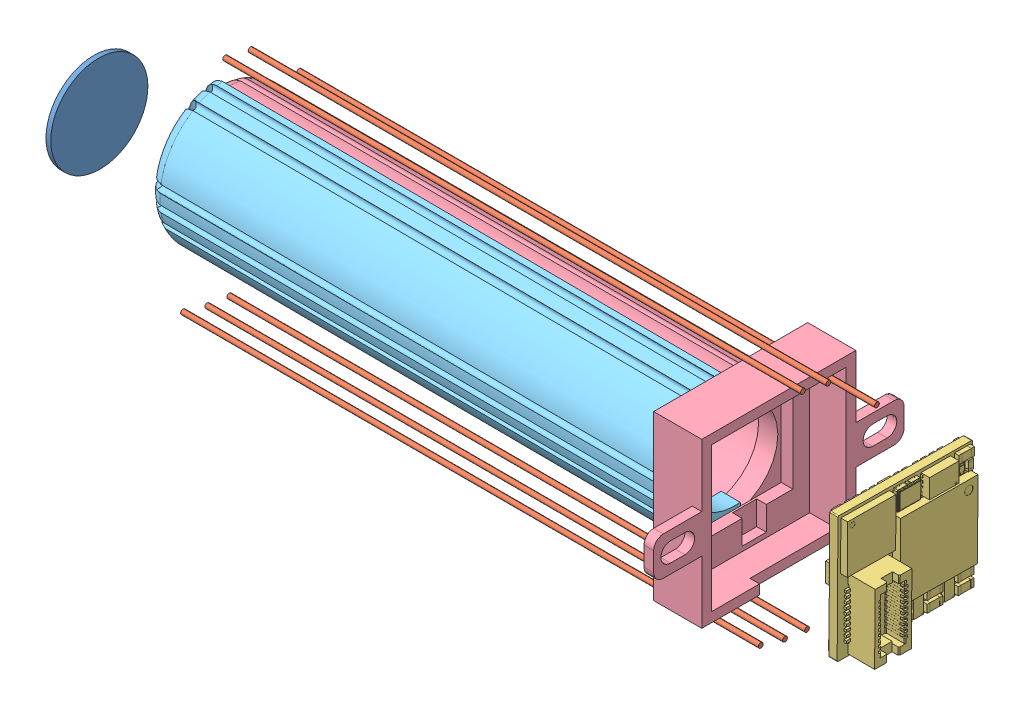
SolidWorks assembly Assem_partialassembled_20241120, configuration Default. Lengths in mm.
Overall size (82.76 21.8 26).
10 component instances, 5 part files, 0 mates.
Components (placement in the parent):
- window-1: window [Default] at (-5.2253 10.4769 -3.9502) x (0.006768 -0.999466 -0.031967) z (-0.008021 -0.03202 0.999455) size (10 0.5 10)
- fiber-1: fiber [Default] at (31.9759 -3.4752 0.5208) size (60 0.5 0.5)
- fiber-2: fiber [Default] at (31.2131 -5.208 -5.0392) size (60 0.5 0.5)
- fiber-3: fiber [Default] at (31.7923 -4.3652 -2.1778) size (60 0.5 0.5)
- fiber-4: fiber [Default] at (30.8935 16.0871 -4.9342) size (60 0.5 0.5)
- fiber-5: fiber [Default] at (31.3406 15.9526 -7.1311) size (60 0.5 0.5)
- fiber-6: fiber [Default] at (32.3947 12.5369 -11.117) size (60 0.5 0.5)
- MU9-MH-BRD.stp-1: MU9-MH-BRD.stp [Default] at (74.5571 8.608 -8.312) x (-0.005156 0.003988 0.999979) z (0.999983 -0.002731 0.005166) size (13.9 13.11 5.52)
- optics_holder_withcam-p1-0603holes-1: optics_holder_withcam-p1-0603holes [Default] at (19.3005 -1.6732 -10.1938) size (58.82 17 26)
- optics_holder_nocap-p2-0605holes-1: optics_holder_nocap-p2-0605holes [Default] at (19.1509 13.6908 -9.9326) x (0.999986 -0.000505 0.005324) z (0.005345 0.12521 -0.992116) size (53.82 14.99 8.71)
